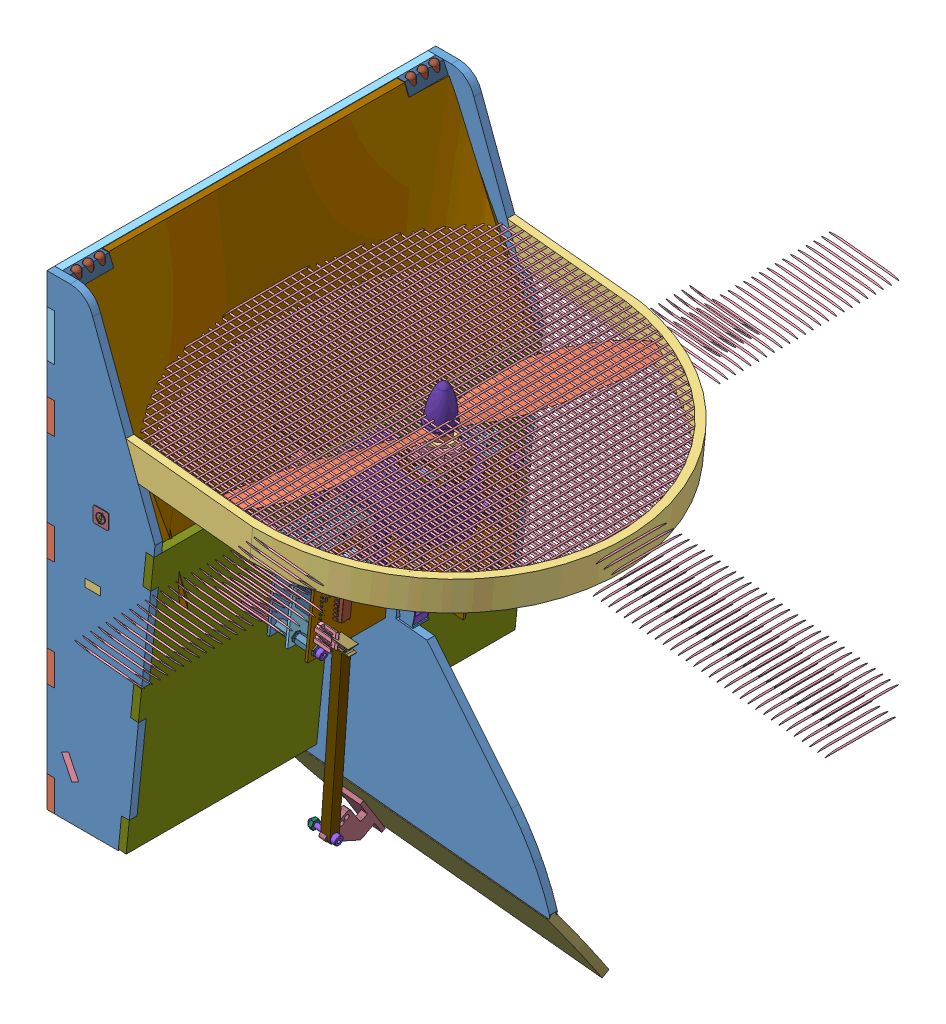
SolidWorks assembly AssTotaleSimu5, configuration Défaut. Lengths in mm. (continued)
Components (placement in the parent): (continued)
- AssStructSimu-1: AssStructSimu [Défaut] at (-125.7658 -1.8483 624.6548) x (1 0 0) z (0 0 -1) size (253.25 324.59 251.6) (continued)
  - AssCarte-1: AssCarte [Défaut] at (38.0121 147.1029 290.772) x (-0.101852 0.9948 0) z (0.9948 0.101852 0) size (66.52 130.57 98.72) (continued)
    - AssEntretoise-3: AssEntretoise [Défaut] at (-106.8199 -51.2976 37.1344) x (0 0 -1) z (1 0 0) size (58.24 7.29 7.81)
      - socket head cap screw 4762_din-1: socket head cap screw 4762_din [EN ISO 4762 M3 x 5 - 5N] at (-2.4967 0.5867 0) size (8 5.5 5.5)
      - hexagonal_spacer_MF_M3_H20_HEX5.5_FTD6_MTL6-1: hexagonal_spacer_MF_M3_H20_HEX5.5_FTD6_MTL6 [Défaut] at (48.3433 0.5867 0) x (0 0 1) z (-1 0 0) size (6.36 5.51 26)
      - hex nut style 1 gradeab_din-1: hex nut style 1 gradeab_din [Hexagon Nut ISO 4032 - M3 - W - N] at (53.3433 0.5867 0) x (0 0.943962 0.330053) z (-1 0 0) size (5.5 6.35 2.4)
      - hexagonal_spacer_MF_M3_H12_HEX5.5_FTD6_MTL6-2: hexagonal_spacer_MF_M3_H12_HEX5.5_FTD6_MTL6 [Défaut] at (27.0633 0.5867 0) x (0 0.248308 0.968681) z (-1 0 0) size (6.36 5.51 18)
      - hexagonal_spacer_MF_M3_H12_HEX5.5_FTD6_MTL6-3: hexagonal_spacer_MF_M3_H12_HEX5.5_FTD6_MTL6 [Défaut] at (13.7833 0.5867 0) x (0 0 1) z (-1 0 0) size (6.36 5.51 18)
    - AssEntretoise-4: AssEntretoise [Défaut] at (-106.8199 68.7024 37.1344) x (0 0 -1) z (1 0 0) size (58.24 7.29 7.81)
      - socket head cap screw 4762_din-1: socket head cap screw 4762_din [EN ISO 4762 M3 x 5 - 5N] at (-2.4967 0.5867 0) size (8 5.5 5.5)
      - hexagonal_spacer_MF_M3_H20_HEX5.5_FTD6_MTL6-1: hexagonal_spacer_MF_M3_H20_HEX5.5_FTD6_MTL6 [Défaut] at (48.3433 0.5867 0) x (0 0 1) z (-1 0 0) size (6.36 5.51 26)
      - hex nut style 1 gradeab_din-1: hex nut style 1 gradeab_din [Hexagon Nut ISO 4032 - M3 - W - N] at (53.3433 0.5867 0) x (0 0.943962 0.330053) z (-1 0 0) size (5.5 6.35 2.4)
      - hexagonal_spacer_MF_M3_H12_HEX5.5_FTD6_MTL6-2: hexagonal_spacer_MF_M3_H12_HEX5.5_FTD6_MTL6 [Défaut] at (27.0633 0.5867 0) x (0 0.248308 0.968681) z (-1 0 0) size (6.36 5.51 18)
      - hexagonal_spacer_MF_M3_H12_HEX5.5_FTD6_MTL6-3: hexagonal_spacer_MF_M3_H12_HEX5.5_FTD6_MTL6 [Défaut] at (13.7833 0.5867 0) x (0 0 1) z (-1 0 0) size (6.36 5.51 18)
    - AssMpu-1: AssMpu [Défaut] at (-150.6881 40.5798 29.6372) x (0.908747 0.417347 0) z (0 0 1) size (8 8 22.28)
      - hex nut style 1 gradeab_din-1: hex nut style 1 gradeab_din [Hexagon Nut ISO 4032 - M3 - W - N] at (0.2783 0.3227 1.2) size (5.5 6.35 2.4)
      - plain washer 6903 type ab_din-1: plain washer 6903 type ab_din [DIN 6903-A3] at (0.2783 0.3227 1.2) x (0 0 1) z (-1 0 0) size (1 8 8)
      - socket head cap screw 4762_din-1: socket head cap screw 4762_din [EN ISO 4762 M3 x 5 - 5N] at (0.2783 0.3227 19.76) x (0 0 -1) z (-0.852155 0.523289 0) size (8 5.5 5.5)
      - hexagonal_spacer_MF_M3_H12_HEX5.5_FTD6_MTL6-1: hexagonal_spacer_MF_M3_H12_HEX5.5_FTD6_MTL6 [Défaut] at (0.2783 0.3227 3.48) size (6.36 5.51 18)
    - AssMpu-2: AssMpu [Défaut] at (-130.3481 40.6665 29.6372) size (8 8 22.28)
      - hex nut style 1 gradeab_din-1: hex nut style 1 gradeab_din [Hexagon Nut ISO 4032 - M3 - W - N] at (0.2783 0.3227 1.2) size (5.5 6.35 2.4)
      - plain washer 6903 type ab_din-1: plain washer 6903 type ab_din [DIN 6903-A3] at (0.2783 0.3227 1.2) x (0 0 1) z (-1 0 0) size (1 8 8)
      - socket head cap screw 4762_din-1: socket head cap screw 4762_din [EN ISO 4762 M3 x 5 - 5N] at (0.2783 0.3227 19.76) x (0 0 -1) z (-0.852155 0.523289 0) size (8 5.5 5.5)
      - hexagonal_spacer_MF_M3_H12_HEX5.5_FTD6_MTL6-1: hexagonal_spacer_MF_M3_H12_HEX5.5_FTD6_MTL6 [Défaut] at (0.2783 0.3227 3.48) size (6.36 5.51 18)
    - AssCosse-1: AssCosse [Défaut] at (-142.6764 26.8797 71.168) x (0 -1 0) z (-0.344896 0 -0.938641) size (9.83 18.66 11.64)
      - socket head cap screw 4762_din-1: socket head cap screw 4762_din [EN ISO 4762 M3 x 6 - 6N] at (-5.1064 0.3659 0) size (9 5.5 5.5)
      - plain washer 6903 type ab_din-1: plain washer 6903 type ab_din [DIN 6903-A3] at (-2.1064 0.3659 0) size (1 8 8)
      - hex nut style 1 gradeab_din-2: hex nut style 1 gradeab_din [Hexagon Nut ISO 4032 - M3 - W - N] at (1.281 0.3659 0) x (0 0.924225 0.381849) z (-1 0 0) size (5.5 6.35 2.4)
      - 31880-1: 31880 [Default] at (0.4936 0.3659 0) x (0 0.344896 -0.938641) z (0 -0.938641 -0.344896) size (5.54 5 17.37)
    - AssCosse-2: AssCosse [Défaut] at (-142.6764 -2.9203 71.168) x (0 -1 0) z (-0.344896 0 -0.938641) size (9.83 18.66 11.64)
      - socket head cap screw 4762_din-1: socket head cap screw 4762_din [EN ISO 4762 M3 x 6 - 6N] at (-5.1064 0.3659 0) size (9 5.5 5.5)
      - plain washer 6903 type ab_din-1: plain washer 6903 type ab_din [DIN 6903-A3] at (-2.1064 0.3659 0) size (1 8 8)
      - hex nut style 1 gradeab_din-2: hex nut style 1 gradeab_din [Hexagon Nut ISO 4032 - M3 - W - N] at (1.281 0.3659 0) x (0 0.924225 0.381849) z (-1 0 0) size (5.5 6.35 2.4)
      - 31880-1: 31880 [Default] at (0.4936 0.3659 0) x (0 0.344896 -0.938641) z (0 -0.938641 -0.344896) size (5.54 5 17.37)
    - AssCosse-3: AssCosse [Défaut] at (-142.6764 12.0797 71.168) x (0 -1 0) z (-0.344896 0 -0.938641) size (9.83 18.66 11.64)
      - socket head cap screw 4762_din-1: socket head cap screw 4762_din [EN ISO 4762 M3 x 6 - 6N] at (-5.1064 0.3659 0) size (9 5.5 5.5)
      - plain washer 6903 type ab_din-1: plain washer 6903 type ab_din [DIN 6903-A3] at (-2.1064 0.3659 0) size (1 8 8)
      - hex nut style 1 gradeab_din-2: hex nut style 1 gradeab_din [Hexagon Nut ISO 4032 - M3 - W - N] at (1.281 0.3659 0) x (0 0.924225 0.381849) z (-1 0 0) size (5.5 6.35 2.4)
      - 31880-1: 31880 [Default] at (0.4936 0.3659 0) x (0 0.344896 -0.938641) z (0 -0.938641 -0.344896) size (5.54 5 17.37)
    - Terminal_QD_Female-1: Terminal_QD_Female [Default] at (-137.2199 31.5422 53.3942) x (0 1 0) z (-1 0 0) size (9.4 5.5 22.35)
    - Terminal_QD_Female-2: Terminal_QD_Female [Default] at (-137.3199 31.5422 36.2942) x (0 -1 0) z (-1 0 0) size (9.4 5.5 22.35)
    - Terminal_QD_Female-3: Terminal_QD_Female [Default] at (-137.2199 1.7422 53.3942) x (0 1 0) z (-1 0 0) size (9.4 5.5 22.35)
    - Terminal_QD_Female-4: Terminal_QD_Female [Default] at (-137.3199 1.7422 35.9942) x (0 1 0) z (-1 0 0) size (9.4 5.5 22.35)
    - Terminal_QD_Female-5: Terminal_QD_Female [Default] at (-137.3199 16.7422 35.9942) x (0 1 0) z (-1 0 0) size (9.4 5.5 22.35)
    - Terminal_QD_Female-6: Terminal_QD_Female [Default] at (-137.2199 16.7422 53.3942) x (0 1 0) z (-1 0 0) size (9.4 5.5 22.35)
- AssTige-1: AssTige [Défaut] at (-241.576 -121.7726 340.4233) x (-0.101791 -0.994204 -0.034587) z (0.9948 -0.101852 0) size (166.39 7.19 19)
  - tige_servo-1: tige_servo [Défaut] at (-106.2712 0.2685 162) size (165 6 6)
  - socket head cap screw 4762_din-2: socket head cap screw 4762_din [EN ISO 4762 M2 x 10 - 10N] at (-104.2712 3.2685 170) x (0 0 -1) z (0.923728 0.383049 0) size (12 3.8 3.8)
  - hex nut style 1 gradeab_din-1: hex nut style 1 gradeab_din [Hexagon Nut ISO 4032 - M3 - W - N] at (55.7288 3.2685 156) size (5.5 6.35 2.4)
  - hex nut style 1 gradeab_din-2: hex nut style 1 gradeab_din [Hexagon Nut ISO 4032 - M2 - W - N] at (-104.2712 3.2685 160) x (0.904801 0.425836 0) z (0 0 1) size (4 4.62 1.6)
  - socket head cap screw 4762_din-3: socket head cap screw 4762_din [EN ISO 4762 M3 x 16 - 16N] at (55.7288 3.2685 171) x (0 0 -1) z (0.923728 0.383049 0) size (19 5.5 5.5)
- AssGoPro-1: AssGoPro [Défaut] at (-119.9926 15.1708 318.2917) x (0 0 -1) z (-0.119031 -0.99289 0) size (64.3 52.3 34.42)
  - GoPRo Frame for LCD Screen-1: GoPRo Frame for LCD Screen [Défaut] at (-2.6935 10.9558 5.5635) size (64.3 47.42 34.42)
    - GoProFrame MJM-1: GoProFrame MJM [Défaut] at (-3.6084 -1.6692 52.45) size (64.3 59.3 23.5)
    - GoPro Hero 3 Front Panel-1: GoPro Hero 3 Front Panel [Défaut] at (-3.6084 -1.6692 55.7) x (-1 0 0) z (0 0 -1) size (59.25 41.2 1.9)
    - GoPro Hero 3 Screen-1: GoPro Hero 3 Screen [Défaut] at (12.7166 3.9308 54.9) size (15 18 1)
    - GoPro Hero 3 Mode Button-1: GoPro Hero 3 Mode Button [Défaut] at (13.4166 -12.4692 54.95) x (-1 0 0) z (0 0 -1) size (11.97 12.11 3.03)
    - GoPro Hero 3 LED Cover-1: GoPro Hero 3 LED Cover [Défaut] at (3.1166 -9.3192 54.85) x (-0.999988 0.004848 0) z (0 0 -1) size (5 5 1.4)
    - GoPro Hero 3 LED Cover-2: GoPro Hero 3 LED Cover [Défaut] at (3.1166 -16.0692 54.85) x (-0.999988 0.004848 0) z (0 0 -1) size (5 5 1.4)
    - GoPro Hero 3 Housing-1: GoPro Hero 3 Housing [Défaut] at (-3.6084 -1.6692 55.7) size (59.37 41.3 29.84)
    - GoPro Hero 3 Lens-1: GoPro Hero 3 Lens [Défaut] at (-18.9334 5.6308 47.35) x (-0.380542 -0.924764 0) z (0 0 -1) size (13.71 15.7 7.94)
    - GoPro Hero 3 Indicator Cover-1: GoPro Hero 3 Indicator Cover [Défaut] at (-25.5834 -22.2692 69.9) x (-0.997412 0 -0.0719) z (0 1 0) size (3 3 2)
    - GoPro Hero 3 Indicator Cover-2: GoPro Hero 3 Indicator Cover [Défaut] at (-28.8834 12.2308 73) x (-0.999992 0.004018 0) z (0 0 1) size (3 3 2)
    - GoPro Hero 3 Indicator Cover-3: GoPro Hero 3 Indicator Cover [Défaut] at (20.6666 16.9308 58.4) x (-0.997739 0 -0.067212) z (0 1 0) size (3 3 2)
    - slot-1: slot [Défaut] at (-24.7434 -9.7363 65.05) x (0 1 0) z (0 0 -1) size (16 15.02 2.44)
    - GoPro Hero 3 HDMI pin-1: GoPro Hero 3 HDMI pin [Défaut] at (-26.982 2.9815 24.7172) x (0.105491 0.98175 -0.158237) z (-0.992872 0.095109 -0.071829) size (3.29 0.86 3.28)
  - support1-2: support1 [Défaut] at (-1.3019 -18.8633 67.0135) x (0 0 1) z (-1 0 0) size (5 5 10)
- AssGouv-1: AssGouv [Défaut] at (-43.2668 -298.2106 479.8345) x (0.9948 -0.101852 0) z (0.055947 0.546439 -0.835628) size (200.18 52.5 43.47)
  - P10_1-1: P10_1 [Défaut] at (-108.1667 -19.4144 197.6829) size (200.18 50.13 5)
  - attache_pale-1: attache_pale [Défaut] at (-49.1667 8.0856 190.1829) x (0 0 -1) z (-1 0 0) size (43.47 35 14)
- Parallax-Servo-Horn-1: Parallax-Servo-Horn [Défaut] at (-69.3162 -29.8353 324.5606) x (0.09792 0.956393 0.27518) z (0.9948 -0.101852 0) size (38.81 38.81 6.17)
- NTM_35-36_engine_assembly-1: NTM_35-36_engine_assembly [Défaut] at (-24.3523 26.8781 325.7101) x (0.9948 -0.101852 0) z (0 0 1) size (60.56 77.2 246.41)
  - engine_base-1: engine_base [Défaut] at (-1.8719 -19.5526 -1.1165) x (0 1 0) z (0 0 1) size (6.8 35 35)
  - engine_bearing-1: engine_bearing [Défaut] at origin size (10 4 10)
  - Propeller_cone-1: Propeller_cone [Défaut] at (-1.8719 33.6474 -4.1165) x (1 0 0) z (0 1 0) size (17.6 17.6 24)
  - engine_bearing-2: engine_bearing [Défaut] at (0 22.8 0) size (10 4 10)
  - NTM_35-36_enginebody-1: NTM_35-36_enginebody [Défaut] at (-1.8719 -12.7526 -1.1165) size (35 31.7 35)
  - Stator-1: Stator [Défaut] at origin size (27.75 22.36 27.94)
  - propellers_10x4-1: propellers_10x4 [Défaut] at (-6.8719 27.4474 -4.9165) size (60.56 10.53 246.41)
  - propeller_washer-1: propeller_washer [Défaut] at (-1.8719 24.4474 -1.1165) x (0 1 0) z (0 0 1) size (2.5 18 18)
  - Propeller_adaptor-1: Propeller_adaptor [Défaut] at (2.1948 17.1101 -3.713) size (23.46 32.5 25)
Mates (geometry in assembly coordinates):
- Coaxiale1: concentric aligned: cylinder of AssStructSimu-1/AssToitMot-1/AssToit-1/P12-1 through (-27.6967 12.5918 324.5936) axis (-0.101852 -0.9948 0) radius 17.5; cylinder of NTM_35-36_engine_assembly-1/NTM_35-36_enginebody-1 through (-25.2217 36.7654 324.5936) axis (-0.101852 -0.9948 0) radius 17.5
- Coïncidente1: coincident anti-aligned: plane of AssStructSimu-1/AssToitMot-1/AssToit-1/P12-1 through (-28.206 7.6178 324.5936) normal (0.101852 0.9948 0); plane of NTM_35-36_engine_assembly-1/engine_bearing-1 through (-28.206 7.6178 324.5936) normal (-0.101852 -0.9948 0)
- Coaxiale2: concentric aligned: cylinder of AssStructSimu-1/AssToitMot-1/AssToit-1/P10_2-1 through (49.7135 -178.7878 324.5936) axis (-0.9948 0.101852 0) radius 2.5; cylinder of AssGouv-1/P10_1-1 through (-94.0351 -164.0702 324.5936) axis (-0.9948 0.101852 0) radius 2.5
- Coïncidente2: coincident aligned: plane of AssStructSimu-1/AssToitMot-1/AssToit-1/P10_2-1 through (-137.5516 -157.1017 322.0936) normal (-0.9948 0.101852 0); plane of AssGouv-1/P10_1-1 through (-137.8791 -160.3008 321.1312) normal (-0.9948 0.101852 0)
- Coaxiale3: concentric aligned: cylinder of AssTige-1/socket head cap screw 4762_din-3 through (-45.5416 -197.7164 335.2292) axis (0.9948 -0.101852 0) radius 1.5; cylinder of AssGouv-1/attache_pale-1 through (-85.9983 -193.5742 335.2292) axis (0.9948 -0.101852 0) radius 1.5
- Coaxiale4: concentric aligned: cylinder of AssStructSimu-1/AssToitMot-1/Parallax-Servo_DUMMY-1 through (-70.6554 -29.6982 324.5606) axis (-0.9948 0.101852 0) radius 2.9845; cylinder of Parallax-Servo-Horn-1 through (-70.6554 -29.6982 324.5606) axis (-0.9948 0.101852 0) radius 2.9845
- Coïncidente3: coincident anti-aligned: plane of AssStructSimu-1/AssToitMot-1/Parallax-Servo_DUMMY-1 through (-74.8246 -29.2713 324.5606) normal (0.9948 -0.101852 0); plane of Parallax-Servo-Horn-1 through (-74.8246 -29.2713 324.5606) normal (-0.9948 0.101852 0)
- Coaxiale5: concentric anti-aligned: cylinder of AssTige-1/socket head cap screw 4762_din-2 through (-30.2498 -38.5418 340.7631) axis (0.9948 -0.101852 0) radius 1; cylinder of Parallax-Servo-Horn-1 through (-69.7931 -34.4932 340.7631) axis (-0.9948 0.101852 0) radius 0.635
- Coïncidente4: coincident anti-aligned: plane of AssTige-1/tige_servo-1 through (-69.6001 -32.608 343.8305) normal (-0.9948 0.101852 0); plane of Parallax-Servo-Horn-1 through (-68.8748 -25.5237 332.3708) normal (0.9948 -0.101852 0)
- Coaxiale6: concentric aligned: cylinder of AssStructSimu-1/AssBase-1/socket head cap screw 4762_din-7 through (-144.5139 -51.9008 369.3436) axis (0 0 1) radius 1.5; cylinder of AssGoPro-1/support1-2 through (-144.5139 -51.9008 319.5936) axis (0 0 1) radius 1.5
- Coïncidente5: coincident anti-aligned: plane of AssStructSimu-1/AssBase-1/support2-1 through (-141.9706 -54.3568 329.5936) normal (0 0 -1); plane of AssGoPro-1/support1-2 through (-146.6985 -49.121 329.5936) normal (0 0 1)
